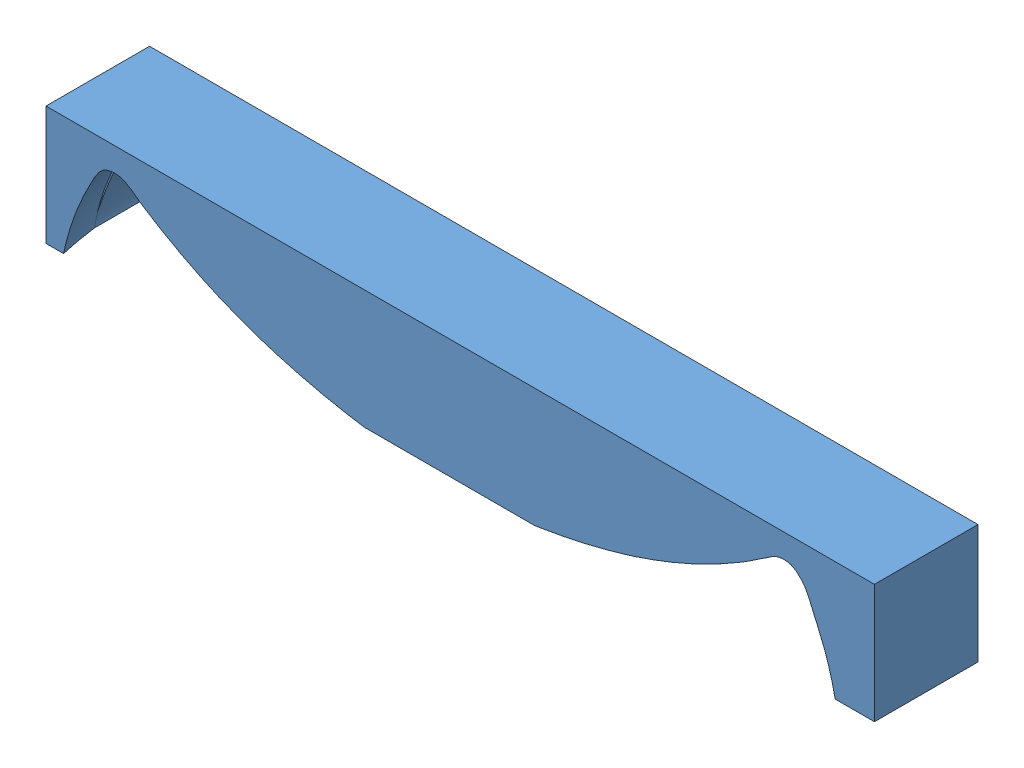
SolidWorks assembly Cutter Assembly, configuration Default. Lengths in mm.
Overall size (80 52.44 12.36).
2 component instances, 2 part files, 0 mates.
Components (placement in the parent):
- UrinDX Housing-1: UrinDX Housing [Default] at (-11.1137 41.6706 122.5778) size (92.88 99.26 108.22) (hidden)
- Attachment Interface-1: Attachment Interface [Default] at (-15.1424 124.8418 50.2179) x (1 0 0) z (0 -1 0) size (80 12.36 13.94)
